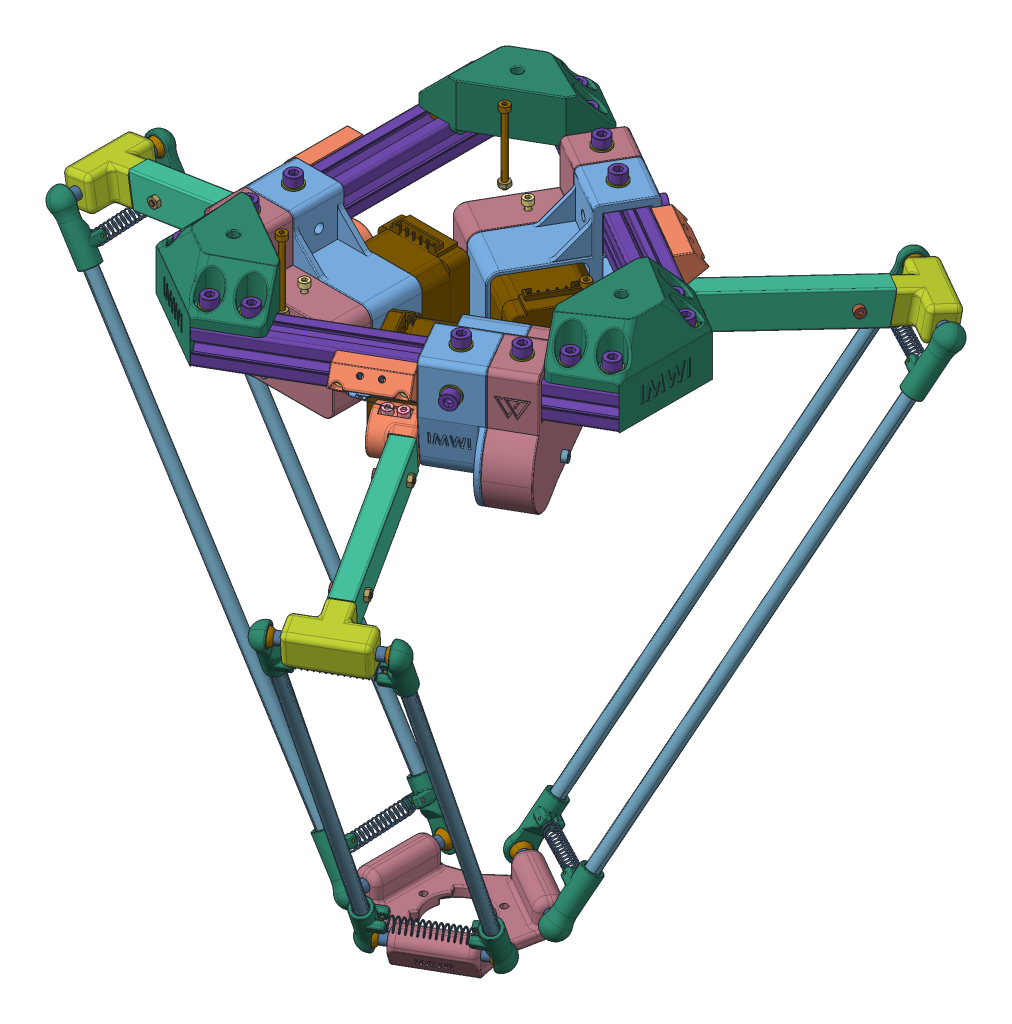
SolidWorks assembly Delta X 1 - v2, configuration 默认. Lengths in mm.
Overall size (365.97 369.79 411.99).
296 component instances, 48 part files, 0 mates.
Components (placement in the parent):
- Delta X 1 - v2.STEP-1: Delta X 1 - v2.STEP [默认] at origin size (365.97 369.79 411.99)
  - Outer Arm.STEP-1: Outer Arm.STEP [默认] at (231.4137 119.905 169.256) x (0.493973 -0.154803 0.855586) z (-0.077402 -0.987945 -0.134064) size (150 86.45 25.5)
    - inox8.STEP-1: inox8.STEP [默认] at (18.6919 -1.6129 59.7906) size (8 70 8)
    - Shoulder.STEP-1: Shoulder.STEP [默认] at (18.6919 46.2871 59.7906) x (0 0 -1) z (0 1 0) size (24 54 22.11)
    - Nut m3.STEP-1: Nut m3.STEP [默认] at (18.6919 61.3871 54.0406) x (0.866025 -0.5 0) z (-0.5 -0.866025 0) size (7.37 2.8 5.8)
    - Nut m3.STEP-2: Nut m3.STEP [默认] at (18.6919 54.3871 54.0406) x (0.99558 -0.093914 0) z (-0.093914 -0.99558 0) size (7.37 2.8 5.8)
    - M3x8 bolt_M3x8 bolt.STEP-1: M3x8 bolt_M3x8 bolt.STEP [默认] at (18.6919 61.3871 46.2906) x (0 0 1) z (-1 0 0) size (11 5.5 5.5)
    - M3x8 bolt_M3x8 bolt.STEP-2: M3x8 bolt_M3x8 bolt.STEP [默认] at (18.6919 54.3871 46.2906) x (0 0 1) z (-1 0 0) size (11 5.5 5.5)
    - ring 8mm.STEP-1: ring 8mm.STEP [默认] at (18.6919 45.2871 59.7906) size (10.45 1 10.45)
    - Nhomtay_Default_As Machined_.STEP-1: Nhomtay_Default_As Machined_.STEP [默认] at (130.6919 51.8371 59.7906) x (0 0 1) z (0 -1 0) size (20 100 12)
    - ElbowV2.STEP-1: ElbowV2.STEP [默认] at (130.6919 51.8371 50.3406) x (0 -1 0) z (0 0 1) size (40 52 18.92)
    - M4x60 thread_M4x60 thread.STEP-1: M4x60 thread_M4x60 thread.STEP [默认] at (148.6919 96.8371 59.7906) x (0 -1 0) z (0 0 1) size (58 4 4)
    - Joint Ball.STEP-1: Joint Ball.STEP [默认] at (148.6919 79.8371 59.7906) x (0 -1 0) z (-0.713634 0 0.700519) size (9 10 10)
    - vongdem3m.STEP-1: vongdem3m.STEP [默认] at (148.6919 71.8371 59.7906) x (0.999724 0 -0.023481) z (0 1 0) size (6.4 6.4 4)
    - Joint Ball.STEP-2: Joint Ball.STEP [默认] at (148.6919 23.8371 59.7906) x (0 1 0) z (0.144688 0 0.989477) size (9 10 10)
    - vongdem3m.STEP-2: vongdem3m.STEP [默认] at (148.6919 27.8371 59.7906) x (0.999724 0 -0.023481) z (0 1 0) size (6.4 6.4 4)
    - M3x15 bolt_M3x8 bolt.STEP-1: M3x15 bolt_M3x8 bolt.STEP [默认] at (45.6919 60.8371 59.7906) x (0 -1 0) z (0 0 1) size (18 5.5 5.5)
    - M3x15 bolt_M3x8 bolt.STEP-2: M3x15 bolt_M3x8 bolt.STEP [默认] at (115.6919 60.8371 59.7906) x (0 -1 0) z (0 0 1) size (18 5.5 5.5)
    - M3 Nut_M3 Nut.STEP-1: M3 Nut_M3 Nut.STEP [默认] at (45.6919 43.4371 59.7906) x (1 0 0) z (0 -1 0) size (5.5 6.35 2.4)
    - M3 Nut_M3 Nut.STEP-2: M3 Nut_M3 Nut.STEP [默认] at (115.6919 43.4371 59.7906) x (1 0 0) z (0 -1 0) size (5.5 6.35 2.4)
  - Outer Arm.STEP-2: Outer Arm.STEP [默认] at (141.6292 119.905 55.839) x (0.493973 -0.154803 -0.855586) z (-0.077402 -0.987945 0.134064) size (150 86.45 25.5)
    - inox8.STEP-1: inox8.STEP [默认] at (18.6919 -1.6129 59.7906) size (8 70 8)
    - Shoulder.STEP-1: Shoulder.STEP [默认] at (18.6919 46.2871 59.7906) x (0 0 -1) z (0 1 0) size (24 54 22.11)
    - Nut m3.STEP-1: Nut m3.STEP [默认] at (18.6919 61.3871 54.0406) x (0.866025 -0.5 0) z (-0.5 -0.866025 0) size (7.37 2.8 5.8)
    - Nut m3.STEP-2: Nut m3.STEP [默认] at (18.6919 54.3871 54.0406) x (0.99558 -0.093914 0) z (-0.093914 -0.99558 0) size (7.37 2.8 5.8)
    - M3x8 bolt_M3x8 bolt.STEP-1: M3x8 bolt_M3x8 bolt.STEP [默认] at (18.6919 61.3871 46.2906) x (0 0 1) z (-1 0 0) size (11 5.5 5.5)
    - M3x8 bolt_M3x8 bolt.STEP-2: M3x8 bolt_M3x8 bolt.STEP [默认] at (18.6919 54.3871 46.2906) x (0 0 1) z (-1 0 0) size (11 5.5 5.5)
    - ring 8mm.STEP-1: ring 8mm.STEP [默认] at (18.6919 45.2871 59.7906) size (10.45 1 10.45)
    - Nhomtay_Default_As Machined_.STEP-1: Nhomtay_Default_As Machined_.STEP [默认] at (130.6919 51.8371 59.7906) x (0 0 1) z (0 -1 0) size (20 100 12)
    - ElbowV2.STEP-1: ElbowV2.STEP [默认] at (130.6919 51.8371 50.3406) x (0 -1 0) z (0 0 1) size (40 52 18.92)
    - M4x60 thread_M4x60 thread.STEP-1: M4x60 thread_M4x60 thread.STEP [默认] at (148.6919 96.8371 59.7906) x (0 -1 0) z (0 0 1) size (58 4 4)
    - Joint Ball.STEP-1: Joint Ball.STEP [默认] at (148.6919 79.8371 59.7906) x (0 -1 0) z (-0.713634 0 0.700519) size (9 10 10)
    - vongdem3m.STEP-1: vongdem3m.STEP [默认] at (148.6919 71.8371 59.7906) x (0.999724 0 -0.023481) z (0 1 0) size (6.4 6.4 4)
    - Joint Ball.STEP-2: Joint Ball.STEP [默认] at (148.6919 23.8371 59.7906) x (0 1 0) z (0.144688 0 0.989477) size (9 10 10)
    - vongdem3m.STEP-2: vongdem3m.STEP [默认] at (148.6919 27.8371 59.7906) x (0.999724 0 -0.023481) z (0 1 0) size (6.4 6.4 4)
    - M3x15 bolt_M3x8 bolt.STEP-1: M3x15 bolt_M3x8 bolt.STEP [默认] at (45.6919 60.8371 59.7906) x (0 -1 0) z (0 0 1) size (18 5.5 5.5)
    - M3x15 bolt_M3x8 bolt.STEP-2: M3x15 bolt_M3x8 bolt.STEP [默认] at (115.6919 60.8371 59.7906) x (0 -1 0) z (0 0 1) size (18 5.5 5.5)
    - M3 Nut_M3 Nut.STEP-1: M3 Nut_M3 Nut.STEP [默认] at (45.6919 43.4371 59.7906) x (1 0 0) z (0 -1 0) size (5.5 6.35 2.4)
    - M3 Nut_M3 Nut.STEP-2: M3 Nut_M3 Nut.STEP [默认] at (115.6919 43.4371 59.7906) x (1 0 0) z (0 -1 0) size (5.5 6.35 2.4)
  - Outer Arm.STEP-3: Outer Arm.STEP [默认] at (88.2995 119.905 190.3032) x (-0.987945 -0.154803 0) z (0.154803 -0.987945 0) size (150 86.45 25.5)
    - inox8.STEP-1: inox8.STEP [默认] at (18.6919 -1.6129 59.7906) size (8 70 8)
    - Shoulder.STEP-1: Shoulder.STEP [默认] at (18.6919 46.2871 59.7906) x (0 0 -1) z (0 1 0) size (24 54 22.11)
    - Nut m3.STEP-1: Nut m3.STEP [默认] at (18.6919 61.3871 54.0406) x (0.866025 -0.5 0) z (-0.5 -0.866025 0) size (7.37 2.8 5.8)
    - Nut m3.STEP-2: Nut m3.STEP [默认] at (18.6919 54.3871 54.0406) x (0.99558 -0.093914 0) z (-0.093914 -0.99558 0) size (7.37 2.8 5.8)
    - M3x8 bolt_M3x8 bolt.STEP-1: M3x8 bolt_M3x8 bolt.STEP [默认] at (18.6919 61.3871 46.2906) x (0 0 1) z (-1 0 0) size (11 5.5 5.5)
    - M3x8 bolt_M3x8 bolt.STEP-2: M3x8 bolt_M3x8 bolt.STEP [默认] at (18.6919 54.3871 46.2906) x (0 0 1) z (-1 0 0) size (11 5.5 5.5)
    - ring 8mm.STEP-1: ring 8mm.STEP [默认] at (18.6919 45.2871 59.7906) size (10.45 1 10.45)
    - Nhomtay_Default_As Machined_.STEP-1: Nhomtay_Default_As Machined_.STEP [默认] at (130.6919 51.8371 59.7906) x (0 0 1) z (0 -1 0) size (20 100 12)
    - ElbowV2.STEP-1: ElbowV2.STEP [默认] at (130.6919 51.8371 50.3406) x (0 -1 0) z (0 0 1) size (40 52 18.92)
    - M4x60 thread_M4x60 thread.STEP-1: M4x60 thread_M4x60 thread.STEP [默认] at (148.6919 96.8371 59.7906) x (0 -1 0) z (0 0 1) size (58 4 4)
    - Joint Ball.STEP-1: Joint Ball.STEP [默认] at (148.6919 79.8371 59.7906) x (0 -1 0) z (-0.713634 0 0.700519) size (9 10 10)
    - vongdem3m.STEP-1: vongdem3m.STEP [默认] at (148.6919 71.8371 59.7906) x (0.999724 0 -0.023481) z (0 1 0) size (6.4 6.4 4)
    - Joint Ball.STEP-2: Joint Ball.STEP [默认] at (148.6919 23.8371 59.7906) x (0 1 0) z (0.144688 0 0.989477) size (9 10 10)
    - vongdem3m.STEP-2: vongdem3m.STEP [默认] at (148.6919 27.8371 59.7906) x (0.999724 0 -0.023481) z (0 1 0) size (6.4 6.4 4)
    - M3x15 bolt_M3x8 bolt.STEP-1: M3x15 bolt_M3x8 bolt.STEP [默认] at (45.6919 60.8371 59.7906) x (0 -1 0) z (0 0 1) size (18 5.5 5.5)
    - M3x15 bolt_M3x8 bolt.STEP-2: M3x15 bolt_M3x8 bolt.STEP [默认] at (115.6919 60.8371 59.7906) x (0 -1 0) z (0 0 1) size (18 5.5 5.5)
    - M3 Nut_M3 Nut.STEP-1: M3 Nut_M3 Nut.STEP [默认] at (45.6919 43.4371 59.7906) x (1 0 0) z (0 -1 0) size (5.5 6.35 2.4)
    - M3 Nut_M3 Nut.STEP-2: M3 Nut_M3 Nut.STEP [默认] at (115.6919 43.4371 59.7906) x (1 0 0) z (0 -1 0) size (5.5 6.35 2.4)
  - MovingBase.STEP-1: MovingBase.STEP [默认] at (35.2258 -322.437 -163.4216) x (0.349728 0 0.936851) z (0 1 0) size (119.04 117.52 20.05)
    - Base-EndEffecterV2.STEP-1: Base-EndEffecterV2.STEP [默认] at (324.2859 5.4897 79.9169) x (0.771299 0.636473 0) z (0 0 1) size (89.65 78.39 20.05)
    - Joint Ball.STEP-1: Joint Ball.STEP [默认] at (338.4028 -36.7562 92.9169) x (-0.936851 0.349728 0) z (-0.29757 -0.79713 0.525391) size (9 10 10)
    - Joint Ball.STEP-2: Joint Ball.STEP [默认] at (285.9391 -17.1714 92.9169) x (0.936851 -0.349728 0) z (0 0 1) size (9 10 10)
    - vongdem3m.STEP-1: vongdem3m.STEP [默认] at (334.6554 -35.3573 92.9169) x (0.106119 0.284272 0.952853) z (-0.936851 0.349728 0) size (6.4 6.4 4)
    - vongdem3m.STEP-2: vongdem3m.STEP [默认] at (293.434 -19.9692 92.9169) x (0.09677 0.259227 0.960956) z (-0.936851 0.349728 0) size (6.4 6.4 4)
    - M4x60 thread_M4x60 thread.STEP-1: M4x60 thread_M4x60 thread.STEP [默认] at (267.5294 3.567 92.9169) x (0.771299 0.636473 0) z (0.59811 -0.72481 -0.341927) size (58 4 4)
    - M4x60 thread_M4x60 thread.STEP-2: M4x60 thread_M4x60 thread.STEP [默认] at (350.9991 55.6036 92.9169) x (0.165552 -0.986201 0) z (-0.926759 -0.155574 -0.341927) size (58 4 4)
    - M4x60 thread_M4x60 thread.STEP-3: M4x60 thread_M4x60 thread.STEP [默认] at (354.3293 -42.7016 92.9169) x (-0.936851 0.349728 0) z (0.328649 0.880384 -0.341927) size (58 4 4)
    - vongdem3m.STEP-3: vongdem3m.STEP [默认] at (283.7267 16.9329 92.9169) x (0.193127 -0.234038 0.952853) z (0.771299 0.636473 0) size (6.4 6.4 4)
    - vongdem3m.STEP-4: vongdem3m.STEP [默认] at (354.4757 34.8934 92.9169) x (-0.299246 -0.050234 0.952853) z (0.165552 -0.986201 0) size (6.4 6.4 4)
    - Joint Ball.STEP-3: Joint Ball.STEP [默认] at (280.6415 14.387 92.9169) x (0.771299 0.636473 0) z (-0.54155 0.656269 0.525391) size (9 10 10)
    - Joint Ball.STEP-4: Joint Ball.STEP [默认] at (353.8135 38.8382 92.9169) x (0.165552 -0.986201 0) z (0.83912 0.140862 0.525391) size (9 10 10)
    - vongdem3m.STEP-5: vongdem3m.STEP [默认] at (317.6638 44.9377 92.9169) x (0.176112 -0.213418 0.960956) z (0.771299 0.636473 0) size (6.4 6.4 4)
    - vongdem3m.STEP-6: vongdem3m.STEP [默认] at (361.76 -8.4994 92.9169) x (-0.272882 -0.045808 0.960956) z (0.165552 -0.986201 0) size (6.4 6.4 4)
    - Joint Ball.STEP-5: Joint Ball.STEP [默认] at (323.8342 50.0295 92.9169) x (-0.771299 -0.636473 0) z (0 0 1) size (9 10 10)
    - Joint Ball.STEP-6: Joint Ball.STEP [默认] at (363.0844 -16.3891 92.9169) x (-0.165552 0.986201 0) z (0 0 1) size (9 10 10)
  - OuterArm1.STEP-1: OuterArm1.STEP [默认] at (-114.8621 147.6011 176.4736) x (0 0 1) z (0.53358 -0.845749 0) size (17.15 14.45 330.3)
    - cacbon.STEP-1: cacbon.STEP [默认] at (-10.0075 3.3175 142.8088) size (7 7 286)
    - RodEnd-1-V2.STEP-1: RodEnd-1-V2.STEP [默认] at (-10.0075 3.3175 443.8088) x (1 0 0) z (0 -1 0) size (17.15 37.15 14.3)
    - Spring Stick.STEP-1: Spring Stick.STEP [默认] at (-17.5075 3.3175 423.8089) size (1.5 11.15 1.5)
    - RodEnd-1-V2.STEP-2: RodEnd-1-V2.STEP [默认] at (-10.0075 3.1669 127.8088) x (1 0 0) z (0 1 0) size (17.15 37.15 14.3)
    - Spring Stick.STEP-2: Spring Stick.STEP [默认] at (-17.5075 3.3175 147.8086) size (1.5 11.15 1.5)
  - OuterArm1.STEP-2: OuterArm1.STEP [默认] at (-120.3462 144.1411 100.4586) x (0 0 -1) z (0.53358 -0.845749 0) size (17.15 14.45 330.3)
    - cacbon.STEP-1: cacbon.STEP [默认] at (-10.0075 3.3175 142.8088) size (7 7 286)
    - RodEnd-1-V2.STEP-1: RodEnd-1-V2.STEP [默认] at (-10.0075 3.3175 443.8088) x (1 0 0) z (0 -1 0) size (17.15 37.15 14.3)
    - Spring Stick.STEP-1: Spring Stick.STEP [默认] at (-17.5075 3.3175 423.8089) size (1.5 11.15 1.5)
    - RodEnd-1-V2.STEP-2: RodEnd-1-V2.STEP [默认] at (-10.0075 3.1669 127.8088) x (1 0 0) z (0 1 0) size (17.15 37.15 14.3)
    - Spring Stick.STEP-2: Spring Stick.STEP [默认] at (-17.5075 3.3175 147.8086) size (1.5 11.15 1.5)
  - OuterArm1.STEP-3: OuterArm1.STEP [默认] at (257.9288 144.1411 394.8708) x (-0.866025 0 0.5) z (-0.26679 -0.845749 -0.462094) size (17.15 14.45 330.3)
    - cacbon.STEP-1: cacbon.STEP [默认] at (-10.0075 3.3175 142.8088) size (7 7 286)
    - RodEnd-1-V2.STEP-1: RodEnd-1-V2.STEP [默认] at (-10.0075 3.3175 443.8088) x (1 0 0) z (0 -1 0) size (17.15 37.15 14.3)
    - Spring Stick.STEP-1: Spring Stick.STEP [默认] at (-17.5075 3.3175 423.8089) size (1.5 11.15 1.5)
    - RodEnd-1-V2.STEP-2: RodEnd-1-V2.STEP [默认] at (-10.0075 3.1669 127.8088) x (1 0 0) z (0 1 0) size (17.15 37.15 14.3)
    - Spring Stick.STEP-2: Spring Stick.STEP [默认] at (-17.5075 3.3175 147.8086) size (1.5 11.15 1.5)
  - OuterArm1.STEP-4: OuterArm1.STEP [默认] at (323.7598 144.1411 -79.9311) x (0.866025 0 0.5) z (-0.26679 -0.845749 0.462094) size (17.15 14.45 330.3)
    - cacbon.STEP-1: cacbon.STEP [默认] at (-10.0075 3.3175 142.8088) size (7 7 286)
    - RodEnd-1-V2.STEP-1: RodEnd-1-V2.STEP [默认] at (-10.0075 3.3175 443.8088) x (1 0 0) z (0 -1 0) size (17.15 37.15 14.3)
    - Spring Stick.STEP-1: Spring Stick.STEP [默认] at (-17.5075 3.3175 423.8089) size (1.5 11.15 1.5)
    - RodEnd-1-V2.STEP-2: RodEnd-1-V2.STEP [默认] at (-10.0075 3.1669 127.8088) x (1 0 0) z (0 1 0) size (17.15 37.15 14.3)
    - Spring Stick.STEP-2: Spring Stick.STEP [默认] at (-17.5075 3.3175 147.8086) size (1.5 11.15 1.5)
  - OuterArm1.STEP-5: OuterArm1.STEP [默认] at (321.0177 147.6011 352.1139) x (0.866025 0 -0.5) z (-0.26679 -0.845749 -0.462094) size (17.15 14.45 330.3)
    - cacbon.STEP-1: cacbon.STEP [默认] at (-10.0075 3.3175 142.8088) size (7 7 286)
    - RodEnd-1-V2.STEP-1: RodEnd-1-V2.STEP [默认] at (-10.0075 3.3175 443.8088) x (1 0 0) z (0 -1 0) size (17.15 37.15 14.3)
    - Spring Stick.STEP-1: Spring Stick.STEP [默认] at (-17.5075 3.3175 423.8089) size (1.5 11.15 1.5)
    - RodEnd-1-V2.STEP-2: RodEnd-1-V2.STEP [默认] at (-10.0075 3.1669 127.8088) x (1 0 0) z (0 1 0) size (17.15 37.15 14.3)
    - Spring Stick.STEP-2: Spring Stick.STEP [默认] at (-17.5075 3.3175 147.8086) size (1.5 11.15 1.5)
  - OuterArm1.STEP-6: OuterArm1.STEP [默认] at (255.1868 147.6011 -113.1892) x (-0.866025 0 -0.5) z (-0.26679 -0.845749 0.462094) size (17.15 14.45 330.3)
    - cacbon.STEP-1: cacbon.STEP [默认] at (-10.0075 3.3175 142.8088) size (7 7 286)
    - RodEnd-1-V2.STEP-1: RodEnd-1-V2.STEP [默认] at (-10.0075 3.3175 443.8088) x (1 0 0) z (0 -1 0) size (17.15 37.15 14.3)
    - Spring Stick.STEP-1: Spring Stick.STEP [默认] at (-17.5075 3.3175 423.8089) size (1.5 11.15 1.5)
    - RodEnd-1-V2.STEP-2: RodEnd-1-V2.STEP [默认] at (-10.0075 3.1669 127.8088) x (1 0 0) z (0 1 0) size (17.15 37.15 14.3)
    - Spring Stick.STEP-2: Spring Stick.STEP [默认] at (-17.5075 3.3175 147.8086) size (1.5 11.15 1.5)
  - 2020_Alu profile_Default_As Machined_.STEP-1: 2020_Alu profile_Default_As Machined_.STEP [默认] at (79.0887 91.9416 230.5161) size (20 20 184)
  - Stepper Servo.STEP-1: Stepper Servo.STEP [默认] at (116.6887 57.9416 115.0161) x (-1 0 0) z (0 0 1) size (42.5 46.75 68)
  - GearboxBody V2.STEP-1: GearboxBody V2.STEP [默认] at (79.0887 91.9416 170.0161) size (85.85 74.01 30.29)
  - Alu plate increase hardness.STEP-1: Alu plate increase hardness.STEP [默认] at (79.0887 57.9416 178.0161) x (1 0 0) z (0 1 0) size (80 3 44.3)
  - Cross M3x10 bolt_Cross M3x10 bolt.STEP-1: Cross M3x10 bolt_Cross M3x10 bolt.STEP [默认] at (79.0887 39.3666 179.4161) x (0 0 -1) z (-0.923728 -0.383049 0) size (10 5.5 5.5)
  - Cross M3x10 bolt_Cross M3x10 bolt.STEP-2: Cross M3x10 bolt_Cross M3x10 bolt.STEP [默认] at (79.0887 76.5166 179.4161) x (0 0 -1) z (-0.280639 0.959813 0) size (10 5.5 5.5)
  - M3 Nut_M3 Nut.STEP-1: M3 Nut_M3 Nut.STEP [默认] at (79.0887 76.5166 169.6161) x (0.5 0.866025 0) z (0 0 -1) size (5.5 6.35 2.4)
  - M3 Nut_M3 Nut.STEP-2: M3 Nut_M3 Nut.STEP [默认] at (79.0887 39.3666 169.6161) x (0.5 0.866025 0) z (0 0 -1) size (5.5 6.35 2.4)
  - Bearing 8_16.STEP-1: Bearing 8_16.STEP [默认] at (79.0887 57.9416 172.5161) x (0.889226 0.457467 0) z (0 0 1) size (16 16 5)
  - Bearing 8_16.STEP-2: Bearing 8_16.STEP [默认] at (79.0887 57.9416 147.5161) x (-0.986457 0.164017 0) z (0 0 1) size (16 16 5)
  - Bearing 5_16.STEP-1: Bearing 5_16.STEP [默认] at (107.7439 45.7053 186.7661) x (-0.939098 0.34365 0) z (0 0 1) size (11 11 5)
  - BeltTensioner.STEP-1: BeltTensioner.STEP [默认] at (122.1887 44.4416 192.1661) x (0.999848 0.017452 0) z (0 0 1) size (32.71 12.76 9.8)
  - BeltTensioner2.STEP-1: BeltTensioner2.STEP [默认] at (122.1887 44.4416 192.1661) x (0.999848 0.017452 0) z (0 0 1) size (32.71 12.76 9.8)
  - BeltTensionerBase-v1.STEP-1: BeltTensionerBase-v1.STEP [默认] at (127.3887 57.4416 175.0161) x (0 1 0) z (1 0 0) size (40.1 16.43 24.55)
  - Cross M3x16 bolt_Cross M3x10 bolt.STEP-1: Cross M3x16 bolt_Cross M3x10 bolt.STEP [默认] at (132.1887 42.4416 181.4161) x (0 0 -1) z (0.065564 -0.997848 0) size (16 5.5 5.5)
  - M3x25 bolt_M3x8 bolt.STEP-1: M3x25 bolt_M3x8 bolt.STEP [默认] at (132.1887 73.4416 194.4161) x (0 0 -1) z (1 0 0) size (28 5.5 5.5)
  - M3x12 bolt_M3x8 bolt.STEP-1: M3x12 bolt_M3x8 bolt.STEP [默认] at (107.7439 45.7053 194.6661) x (0 0 -1) z (1 0 0) size (15 5.5 5.5)
  - M3 Nut_M3 Nut.STEP-3: M3 Nut_M3 Nut.STEP [默认] at (107.7439 45.7053 179.4661) x (0.5 0.866025 0) z (0 0 -1) size (5.5 6.35 2.4)
  - M3x20 bolt_M3x8 bolt.STEP-1: M3x20 bolt_M3x8 bolt.STEP [默认] at (122.1887 44.4416 194.6661) x (0 0 -1) z (1 0 0) size (23 5.5 5.5)
  - ring 8mm.STEP-1: ring 8mm.STEP [默认] at (79.0887 57.9416 175.0161) x (1 0 0) z (0 -1 0) size (10.45 1 10.45)
  - GearboxLid V2.STEP-1: GearboxLid V2.STEP [默认] at (79.0887 91.9416 195.4161) size (85.85 74 22.42)
  - M3 Nut_M3 Nut.STEP-4: M3 Nut_M3 Nut.STEP [默认] at (110.9759 77.0916 185.4195) x (1 0 0) z (0 1 0) size (5.5 6.35 2.4)
  - M3x30 bolt_M3x8 bolt.STEP-1: M3x30 bolt_M3x8 bolt.STEP [默认] at (101.1887 42.4416 200.4161) x (0 0 -1) z (1 0 0) size (33 5.5 5.5)
  - M3x30 bolt_M3x8 bolt.STEP-2: M3x30 bolt_M3x8 bolt.STEP [默认] at (101.1887 73.4416 200.4161) x (0 0 -1) z (1 0 0) size (33 5.5 5.5)
  - Frame connector.STEP-1: Frame connector.STEP [默认] at (97.7489 101.9416 235.5161) x (0.866025 0 0.5) z (0 -1 0) size (84.39 40.74 45.28)
  - M5 Washer_M5 Washer.STEP-1: M5 Washer_M5 Washer.STEP [默认] at (131.8474 107.0381 237.3764) x (0 1 0) z (0 0 1) size (1 10 10)
  - M5 Washer_M5 Washer.STEP-2: M5 Washer_M5 Washer.STEP [默认] at (116.2589 106.9416 246.3764) x (0 -1 0) z (0 0 1) size (1 10 10)
  - M5 Washer_M5 Washer.STEP-3: M5 Washer_M5 Washer.STEP [默认] at (79.0887 106.9416 224.9161) x (0 -1 0) z (0 0 1) size (1 10 10)
  - M5 Washer_M5 Washer.STEP-4: M5 Washer_M5 Washer.STEP [默认] at (79.0887 106.9416 206.9161) x (0 -1 0) z (0 0 1) size (1 10 10)
  - M5 Washer_M5 Washer.STEP-5: M5 Washer_M5 Washer.STEP [默认] at (79.0887 106.9416 186.2161) x (0 -1 0) z (0 0 1) size (1 10 10)
  - M5 Washer_M5 Washer.STEP-6: M5 Washer_M5 Washer.STEP [默认] at (79.0887 106.9416 160.0161) x (0 -1 0) z (0.543109 0 -0.839662) size (1 10 10)
  - M5 Washer_M5 Washer.STEP-7: M5 Washer_M5 Washer.STEP [默认] at (64.0887 91.9416 160.0161) size (1 10 10)
  - M5x10 bolt_M5x10 bolt.STEP-1: M5x10 bolt_M5x10 bolt.STEP [默认] at (79.0887 112.9416 224.9161) x (0 -1 0) z (0 0 1) size (15 8.5 8.5)
  - M5x10 bolt_M5x10 bolt.STEP-2: M5x10 bolt_M5x10 bolt.STEP [默认] at (79.0887 112.9416 206.9161) x (0 -1 0) z (0 0 1) size (15 8.5 8.5)
  - M5x10 bolt_M5x10 bolt.STEP-3: M5x10 bolt_M5x10 bolt.STEP [默认] at (79.0887 112.9416 186.2161) x (0 -1 0) z (0 0 1) size (15 8.5 8.5)
  - M5x10 bolt_M5x10 bolt.STEP-4: M5x10 bolt_M5x10 bolt.STEP [默认] at (79.0887 112.9416 160.0161) x (0 -1 0) z (0 0 1) size (15 8.5 8.5)
  - M5x10 bolt_M5x10 bolt.STEP-5: M5x10 bolt_M5x10 bolt.STEP [默认] at (58.0887 91.9416 160.0161) size (15 8.5 8.5)
  - M5x10 bolt_M5x10 bolt.STEP-6: M5x10 bolt_M5x10 bolt.STEP [默认] at (116.2589 112.9416 246.3764) x (0 -1 0) z (0 0 1) size (15 8.5 8.5)
  - M5x10 bolt_M5x10 bolt.STEP-7: M5x10 bolt_M5x10 bolt.STEP [默认] at (131.8474 112.0381 237.3764) x (0 -1 0) z (0 0 1) size (15 8.5 8.5)
  - T Slot Nut_______ _______ 6__ _5.STEP-1: T Slot Nut_______ _______ 6__ _5.STEP [默认] at (79.0887 97.2416 155.0161) size (9.4 4.5 10)
  - T Slot Nut_______ _______ 6__ _5.STEP-2: T Slot Nut_______ _______ 6__ _5.STEP [默认] at (73.7887 91.9416 155.0161) x (0 1 0) z (0 0 1) size (9.4 4.5 10)
  - T Slot Nut_______ _______ 6__ _5.STEP-3: T Slot Nut_______ _______ 6__ _5.STEP [默认] at (79.0887 97.2416 181.2161) size (9.4 4.5 10)
  - T Slot Nut_______ _______ 6__ _5.STEP-4: T Slot Nut_______ _______ 6__ _5.STEP [默认] at (79.0887 97.2416 201.0161) size (9.4 4.5 10)
  - T Slot Nut_______ _______ 6__ _5.STEP-5: T Slot Nut_______ _______ 6__ _5.STEP [默认] at (79.0887 97.2416 219.0161) size (9.4 4.5 10)
  - T Slot Nut_______ _______ 6__ _5.STEP-6: T Slot Nut_______ _______ 6__ _5.STEP [默认] at (128.2967 97.2416 239.4263) x (-0.5 0 -0.866025) z (0.866025 0 -0.5) size (9.4 4.5 10)
  - T Slot Nut_______ _______ 6__ _5.STEP-7: T Slot Nut_______ _______ 6__ _5.STEP [默认] at (112.7082 97.2416 248.4263) x (-0.5 0 -0.866025) z (0.866025 0 -0.5) size (9.4 4.5 10)
  - M3 Nut_M3 Nut.STEP-5: M3 Nut_M3 Nut.STEP [默认] at (212.3063 45.7053 157.8352) x (-0.25 0.866025 -0.433013) z (-0.866025 0 0.5) size (5.5 6.35 2.4)
  - M3 Nut_M3 Nut.STEP-6: M3 Nut_M3 Nut.STEP [默认] at (141.2922 45.7053 78.097) x (-0.25 0.866025 0.433013) z (0.866025 0 0.5) size (5.5 6.35 2.4)
  - Stepper Servo.STEP-2: Stepper Servo.STEP [默认] at (152.0185 57.9416 182.3138) x (0.5 0 0.866025) z (0.866025 0 -0.5) size (42.5 46.75 68)
  - Stepper Servo.STEP-3: Stepper Servo.STEP [默认] at (192.6351 57.9416 118.0684) x (0.5 0 -0.866025) z (-0.866025 0 -0.5) size (42.5 46.75 68)
  - Cross M3x10 bolt_Cross M3x10 bolt.STEP-3: Cross M3x10 bolt_Cross M3x10 bolt.STEP [默认] at (226.5906 76.5166 182.6764) x (-0.866025 0 0.5) z (0.14032 0.959813 0.243041) size (10 5.5 5.5)
  - Cross M3x10 bolt_Cross M3x10 bolt.STEP-4: Cross M3x10 bolt_Cross M3x10 bolt.STEP [默认] at (155.6631 76.5166 53.3058) x (0.866025 0 0.5) z (0.14032 0.959813 -0.243041) size (10 5.5 5.5)
  - T Slot Nut_______ _______ 6__ _5.STEP-8: T Slot Nut_______ _______ 6__ _5.STEP [默认] at (228.1494 97.2416 181.7764) x (-0.5 0 -0.866025) z (0.866025 0 -0.5) size (9.4 4.5 10)
  - T Slot Nut_______ _______ 6__ _5.STEP-9: T Slot Nut_______ _______ 6__ _5.STEP [默认] at (154.1043 97.2416 52.4058) x (-0.5 0 0.866025) z (-0.866025 0 -0.5) size (9.4 4.5 10)
  - T Slot Nut_______ _______ 6__ _5.STEP-10: T Slot Nut_______ _______ 6__ _5.STEP [默认] at (208.1096 91.9416 199.4663) x (0 1 0) z (0.866025 0 -0.5) size (9.4 4.5 10)
  - T Slot Nut_______ _______ 6__ _5.STEP-11: T Slot Nut_______ _______ 6__ _5.STEP [默认] at (179.4441 91.9416 60.9159) x (0 1 0) z (-0.866025 0 -0.5) size (9.4 4.5 10)
  - T Slot Nut_______ _______ 6__ _5.STEP-12: T Slot Nut_______ _______ 6__ _5.STEP [默认] at (260.8852 97.2416 162.8764) x (-0.5 0 -0.866025) z (0.866025 0 -0.5) size (9.4 4.5 10)
  - T Slot Nut_______ _______ 6__ _5.STEP-13: T Slot Nut_______ _______ 6__ _5.STEP [默认] at (121.3685 97.2416 33.5058) x (-0.5 0 0.866025) z (-0.866025 0 -0.5) size (9.4 4.5 10)
  - T Slot Nut_______ _______ 6__ _5.STEP-14: T Slot Nut_______ _______ 6__ _5.STEP [默认] at (253.957 97.2416 110.0558) x (-0.5 0 0.866025) z (-0.866025 0 -0.5) size (9.4 4.5 10)
  - T Slot Nut_______ _______ 6__ _5.STEP-15: T Slot Nut_______ _______ 6__ _5.STEP [默认] at (79.0887 97.2416 65.9161) size (9.4 4.5 10)
  - T Slot Nut_______ _______ 6__ _5.STEP-16: T Slot Nut_______ _______ 6__ _5.STEP [默认] at (269.5454 97.2416 119.0558) x (-0.5 0 0.866025) z (-0.866025 0 -0.5) size (9.4 4.5 10)
  - T Slot Nut_______ _______ 6__ _5.STEP-17: T Slot Nut_______ _______ 6__ _5.STEP [默认] at (79.0887 97.2416 47.9161) size (9.4 4.5 10)
  - T Slot Nut_______ _______ 6__ _5.STEP-18: T Slot Nut_______ _______ 6__ _5.STEP [默认] at (245.2967 97.2416 171.8764) x (-0.5 0 -0.866025) z (0.866025 0 -0.5) size (9.4 4.5 10)
  - T Slot Nut_______ _______ 6__ _5.STEP-19: T Slot Nut_______ _______ 6__ _5.STEP [默认] at (136.9569 97.2416 42.5058) x (-0.5 0 0.866025) z (-0.866025 0 -0.5) size (9.4 4.5 10)
  - BeltTensionerBase-v1.STEP-2: BeltTensionerBase-v1.STEP [默认] at (198.6301 57.4416 143.0473) x (0 1 0) z (-0.5 0 -0.866025) size (40.1 16.43 24.55)
  - BeltTensionerBase-v1.STEP-3: BeltTensionerBase-v1.STEP [默认] at (135.3236 57.4416 97.3349) x (0 1 0) z (-0.5 0 0.866025) size (40.1 16.43 24.55)
  - Alu plate increase hardness.STEP-2: Alu plate increase hardness.STEP [默认] at (225.3781 57.9416 183.3764) x (-0.5 0 -0.866025) z (0 1 0) size (80 3 44.3)
  - Alu plate increase hardness.STEP-3: Alu plate increase hardness.STEP [默认] at (156.8755 57.9416 54.0058) x (-0.5 0 0.866025) z (0 1 0) size (80 3 44.3)
  - M3x20 bolt_M3x8 bolt.STEP-2: M3x20 bolt_M3x8 bolt.STEP [默认] at (218.2475 44.4416 137.7257) x (-0.866025 0 0.5) z (-0.5 0 -0.866025) size (23 5.5 5.5)
  - M3x20 bolt_M3x8 bolt.STEP-3: M3x20 bolt_M3x8 bolt.STEP [默认] at (120.9062 44.4416 83.0065) x (0.866025 0 0.5) z (-0.5 0 0.866025) size (23 5.5 5.5)
  - M3x12 bolt_M3x8 bolt.STEP-2: M3x12 bolt_M3x8 bolt.STEP [默认] at (225.4699 45.7053 150.2352) x (-0.866025 0 0.5) z (-0.5 0 -0.866025) size (15 5.5 5.5)
  - M3x12 bolt_M3x8 bolt.STEP-3: M3x12 bolt_M3x8 bolt.STEP [默认] at (128.1286 45.7053 70.497) x (0.866025 0 0.5) z (-0.5 0 0.866025) size (15 5.5 5.5)
  - GearboxLid V2.STEP-2: GearboxLid V2.STEP [默认] at (240.447 91.9416 174.6764) x (-0.5 0 -0.866025) z (0.866025 0 -0.5) size (85.85 74 22.42)
  - GearboxLid V2.STEP-3: GearboxLid V2.STEP [默认] at (141.8067 91.9416 45.3058) x (-0.5 0 0.866025) z (-0.866025 0 -0.5) size (85.85 74 22.42)
  - ring 8mm.STEP-2: ring 8mm.STEP [默认] at (222.7801 57.9416 184.8764) x (-0.5 0 -0.866025) z (0 -1 0) size (10.45 1 10.45)
  - ring 8mm.STEP-3: ring 8mm.STEP [默认] at (159.4736 57.9416 55.5058) x (-0.5 0 0.866025) z (0 -1 0) size (10.45 1 10.45)
  - Cross M3x10 bolt_Cross M3x10 bolt.STEP-5: Cross M3x10 bolt_Cross M3x10 bolt.STEP [默认] at (226.5906 39.3666 182.6764) x (-0.866025 0 0.5) z (0.461864 -0.383049 0.799972) size (10 5.5 5.5)
  - Cross M3x10 bolt_Cross M3x10 bolt.STEP-6: Cross M3x10 bolt_Cross M3x10 bolt.STEP [默认] at (155.6631 39.3666 53.3058) x (0.866025 0 0.5) z (0.461864 -0.383049 -0.799972) size (10 5.5 5.5)
  - Cross M3x16 bolt_Cross M3x10 bolt.STEP-2: Cross M3x16 bolt_Cross M3x10 bolt.STEP [默认] at (201.7726 42.4416 135.6904) x (-0.866025 0 0.5) z (-0.032782 -0.997848 -0.05678) size (16 5.5 5.5)
  - Cross M3x16 bolt_Cross M3x10 bolt.STEP-3: Cross M3x16 bolt_Cross M3x10 bolt.STEP [默认] at (127.381 42.4416 98.2918) x (0.866025 0 0.5) z (-0.032782 -0.997848 0.05678) size (16 5.5 5.5)
  - GearboxBody V2.STEP-2: GearboxBody V2.STEP [默认] at (218.4499 91.9416 187.3764) x (-0.5 0 -0.866025) z (0.866025 0 -0.5) size (85.85 74.01 30.29)
  - GearboxBody V2.STEP-3: GearboxBody V2.STEP [默认] at (163.8037 91.9416 58.0058) x (-0.5 0 0.866025) z (-0.866025 0 -0.5) size (85.85 74.01 30.29)
  - M3 Nut_M3 Nut.STEP-7: M3 Nut_M3 Nut.STEP [默认] at (218.1035 39.3666 187.5764) x (-0.25 0.866025 -0.433013) z (-0.866025 0 0.5) size (5.5 6.35 2.4)
  - M3 Nut_M3 Nut.STEP-8: M3 Nut_M3 Nut.STEP [默认] at (164.1501 39.3666 58.2058) x (-0.25 0.866025 0.433013) z (0.866025 0 0.5) size (5.5 6.35 2.4)
  - BeltTensioner2.STEP-2: BeltTensioner2.STEP [默认] at (216.0824 44.4416 138.9757) x (-0.499924 0.017452 -0.865894) z (0.866025 0 -0.5) size (32.71 12.76 9.8)
  - BeltTensioner2.STEP-3: BeltTensioner2.STEP [默认] at (123.0713 44.4416 84.2565) x (-0.499924 0.017452 0.865894) z (-0.866025 0 -0.5) size (32.71 12.76 9.8)
  - M3 Nut_M3 Nut.STEP-9: M3 Nut_M3 Nut.STEP [默认] at (218.1035 76.5166 187.5764) x (-0.25 0.866025 -0.433013) z (-0.866025 0 0.5) size (5.5 6.35 2.4)
  - M3 Nut_M3 Nut.STEP-10: M3 Nut_M3 Nut.STEP [默认] at (164.1501 76.5166 58.2058) x (-0.25 0.866025 0.433013) z (0.866025 0 0.5) size (5.5 6.35 2.4)
  - BeltTensioner.STEP-2: BeltTensioner.STEP [默认] at (216.0824 44.4416 138.9757) x (-0.499924 0.017452 -0.865894) z (0.866025 0 -0.5) size (32.71 12.76 9.8)
  - BeltTensioner.STEP-3: BeltTensioner.STEP [默认] at (123.0713 44.4416 84.2565) x (-0.499924 0.017452 0.865894) z (-0.866025 0 -0.5) size (32.71 12.76 9.8)
  - Bearing 5_16.STEP-2: Bearing 5_16.STEP [默认] at (218.6283 45.7053 154.1852) x (0.469549 0.34365 0.813283) z (0.866025 0 -0.5) size (11 11 5)
  - Bearing 5_16.STEP-3: Bearing 5_16.STEP [默认] at (134.9702 45.7053 74.447) x (0.469549 0.34365 -0.813283) z (-0.866025 0 -0.5) size (11 11 5)
  - M3x25 bolt_M3x8 bolt.STEP-2: M3x25 bolt_M3x8 bolt.STEP [默认] at (213.031 73.4416 129.1904) x (-0.866025 0 0.5) z (-0.5 0 -0.866025) size (28 5.5 5.5)
  - M3x25 bolt_M3x8 bolt.STEP-3: M3x25 bolt_M3x8 bolt.STEP [默认] at (116.1227 73.4416 91.7918) x (0.866025 0 0.5) z (-0.5 0 0.866025) size (28 5.5 5.5)
  - M3x30 bolt_M3x8 bolt.STEP-3: M3x30 bolt_M3x8 bolt.STEP [默认] at (233.7271 73.4416 153.0372) x (-0.866025 0 0.5) z (-0.5 0 -0.866025) size (33 5.5 5.5)
  - M3x30 bolt_M3x8 bolt.STEP-4: M3x30 bolt_M3x8 bolt.STEP [默认] at (126.4266 73.4416 61.945) x (0.866025 0 0.5) z (-0.5 0 0.866025) size (33 5.5 5.5)
  - 2020_Alu profile_Default_As Machined_.STEP-2: 2020_Alu profile_Default_As Machined_.STEP [默认] at (270.8445 91.9416 157.1264) x (-0.5 0 -0.866025) z (0.866025 0 -0.5) size (20 20 184)
  - 2020_Alu profile_Default_As Machined_.STEP-3: 2020_Alu profile_Default_As Machined_.STEP [默认] at (111.4092 91.9416 27.7558) x (-0.5 0 0.866025) z (-0.866025 0 -0.5) size (20 20 184)
  - Bearing 8_16.STEP-3: Bearing 8_16.STEP [默认] at (220.615 57.9416 186.1264) x (-0.444613 0.457467 -0.770093) z (0.866025 0 -0.5) size (16 16 5)
  - Bearing 8_16.STEP-4: Bearing 8_16.STEP [默认] at (161.6387 57.9416 56.7558) x (-0.444613 0.457467 0.770093) z (-0.866025 0 -0.5) size (16 16 5)
  - Bearing 8_16.STEP-5: Bearing 8_16.STEP [默认] at (198.9644 57.9416 198.6264) x (0.493229 0.164017 0.854297) z (0.866025 0 -0.5) size (16 16 5)
  - Bearing 8_16.STEP-6: Bearing 8_16.STEP [默认] at (183.2893 57.9416 69.2558) x (0.493229 0.164017 -0.854297) z (-0.866025 0 -0.5) size (16 16 5)
  - M5 Washer_M5 Washer.STEP-8: M5 Washer_M5 Washer.STEP [默认] at (265.9947 106.9416 117.0058) x (0 -1 0) z (0.866025 0 -0.5) size (1 10 10)
  - M5 Washer_M5 Washer.STEP-9: M5 Washer_M5 Washer.STEP [默认] at (79.0887 106.9416 52.0161) x (0 -1 0) z (-0.866025 0 -0.5) size (1 10 10)
  - M5 Washer_M5 Washer.STEP-10: M5 Washer_M5 Washer.STEP [默认] at (265.9947 106.9416 159.9264) x (0 -1 0) z (0.866025 0 -0.5) size (1 10 10)
  - M5 Washer_M5 Washer.STEP-11: M5 Washer_M5 Washer.STEP [默认] at (116.2589 106.9416 30.5558) x (0 -1 0) z (-0.866025 0 -0.5) size (1 10 10)
  - M5 Washer_M5 Washer.STEP-12: M5 Washer_M5 Washer.STEP [默认] at (250.4063 107.0381 108.0058) x (0 1 0) z (0.866025 0 -0.5) size (1 10 10)
  - M5 Washer_M5 Washer.STEP-13: M5 Washer_M5 Washer.STEP [默认] at (79.0887 107.0381 70.0161) x (0 1 0) z (-0.866025 0 -0.5) size (1 10 10)
  - M5 Washer_M5 Washer.STEP-14: M5 Washer_M5 Washer.STEP [默认] at (209.7897 106.9416 192.3764) x (0 -1 0) z (-0.998723 0 -0.050515) size (1 10 10)
  - M5 Washer_M5 Washer.STEP-15: M5 Washer_M5 Washer.STEP [默认] at (172.464 106.9416 63.0058) x (0 -1 0) z (0.455615 0 0.890177) size (1 10 10)
  - M5 Washer_M5 Washer.STEP-16: M5 Washer_M5 Washer.STEP [默认] at (232.4795 106.9416 179.2764) x (0 -1 0) z (0.866025 0 -0.5) size (1 10 10)
  - M5 Washer_M5 Washer.STEP-17: M5 Washer_M5 Washer.STEP [默认] at (149.7741 106.9416 49.9058) x (0 -1 0) z (-0.866025 0 -0.5) size (1 10 10)
  - M5 Washer_M5 Washer.STEP-18: M5 Washer_M5 Washer.STEP [默认] at (217.2897 91.9416 205.3667) x (-0.5 0 -0.866025) z (0.866025 0 -0.5) size (1 10 10)
  - M5 Washer_M5 Washer.STEP-19: M5 Washer_M5 Washer.STEP [默认] at (179.964 91.9416 50.0155) x (-0.5 0 0.866025) z (-0.866025 0 -0.5) size (1 10 10)
  - M5 Washer_M5 Washer.STEP-20: M5 Washer_M5 Washer.STEP [默认] at (250.4063 106.9416 168.9264) x (0 -1 0) z (0.866025 0 -0.5) size (1 10 10)
  - M5 Washer_M5 Washer.STEP-21: M5 Washer_M5 Washer.STEP [默认] at (131.8474 106.9416 39.5558) x (0 -1 0) z (-0.866025 0 -0.5) size (1 10 10)
  - M3x30 bolt_M3x8 bolt.STEP-5: M3x30 bolt_M3x8 bolt.STEP [默认] at (233.7271 42.4416 153.0372) x (-0.866025 0 0.5) z (-0.5 0 -0.866025) size (33 5.5 5.5)
  - M3x30 bolt_M3x8 bolt.STEP-6: M3x30 bolt_M3x8 bolt.STEP [默认] at (126.4266 42.4416 61.945) x (0.866025 0 0.5) z (-0.5 0 0.866025) size (33 5.5 5.5)
  - M5x10 bolt_M5x10 bolt.STEP-8: M5x10 bolt_M5x10 bolt.STEP [默认] at (250.4063 112.0381 108.0058) x (0 -1 0) z (0.866025 0 -0.5) size (15 8.5 8.5)
  - M5x10 bolt_M5x10 bolt.STEP-9: M5x10 bolt_M5x10 bolt.STEP [默认] at (79.0887 112.0381 70.0161) x (0 -1 0) z (-0.866025 0 -0.5) size (15 8.5 8.5)
  - Frame connector.STEP-2: Frame connector.STEP [默认] at (265.8445 101.9416 138.4661) x (0 0 -1) z (0 -1 0) size (84.39 40.74 45.28)
  - Frame connector.STEP-3: Frame connector.STEP [默认] at (97.7489 101.9416 41.4161) x (-0.866025 0 0.5) z (0 -1 0) size (84.39 40.74 45.28)
  - M3 Nut_M3 Nut.STEP-11: M3 Nut_M3 Nut.STEP [默认] at (215.8461 77.0916 152.0596) x (-0.5 0 -0.866025) z (0 1 0) size (5.5 6.35 2.4)
  - M3 Nut_M3 Nut.STEP-12: M3 Nut_M3 Nut.STEP [默认] at (134.5204 77.0916 77.9193) x (-0.5 0 0.866025) z (0 1 0) size (5.5 6.35 2.4)
  - T Slot Nut_______ _______ 6__ _5.STEP-20: T Slot Nut_______ _______ 6__ _5.STEP [默认] at (205.4596 97.2416 194.8764) x (-0.5 0 -0.866025) z (0.866025 0 -0.5) size (9.4 4.5 10)
  - T Slot Nut_______ _______ 6__ _5.STEP-21: T Slot Nut_______ _______ 6__ _5.STEP [默认] at (176.7941 97.2416 65.5058) x (-0.5 0 0.866025) z (-0.866025 0 -0.5) size (9.4 4.5 10)
  - M5x10 bolt_M5x10 bolt.STEP-10: M5x10 bolt_M5x10 bolt.STEP [默认] at (220.2897 91.9416 210.5629) x (-0.5 0 -0.866025) z (0.866025 0 -0.5) size (15 8.5 8.5)
  - M5x10 bolt_M5x10 bolt.STEP-11: M5x10 bolt_M5x10 bolt.STEP [默认] at (182.964 91.9416 44.8193) x (-0.5 0 0.866025) z (-0.866025 0 -0.5) size (15 8.5 8.5)
  - M5x10 bolt_M5x10 bolt.STEP-12: M5x10 bolt_M5x10 bolt.STEP [默认] at (265.9947 112.9416 117.0058) x (0 -1 0) z (0.866025 0 -0.5) size (15 8.5 8.5)
  - M5x10 bolt_M5x10 bolt.STEP-13: M5x10 bolt_M5x10 bolt.STEP [默认] at (79.0887 112.9416 52.0161) x (0 -1 0) z (-0.866025 0 -0.5) size (15 8.5 8.5)
  - M5x10 bolt_M5x10 bolt.STEP-14: M5x10 bolt_M5x10 bolt.STEP [默认] at (209.7897 112.9416 192.3764) x (0 -1 0) z (0.866025 0 -0.5) size (15 8.5 8.5)
  - M5x10 bolt_M5x10 bolt.STEP-15: M5x10 bolt_M5x10 bolt.STEP [默认] at (172.464 112.9416 63.0058) x (0 -1 0) z (-0.866025 0 -0.5) size (15 8.5 8.5)
  - M5x10 bolt_M5x10 bolt.STEP-16: M5x10 bolt_M5x10 bolt.STEP [默认] at (265.9947 112.9416 159.9264) x (0 -1 0) z (0.866025 0 -0.5) size (15 8.5 8.5)
  - M5x10 bolt_M5x10 bolt.STEP-17: M5x10 bolt_M5x10 bolt.STEP [默认] at (116.2589 112.9416 30.5558) x (0 -1 0) z (-0.866025 0 -0.5) size (15 8.5 8.5)
  - M5x10 bolt_M5x10 bolt.STEP-18: M5x10 bolt_M5x10 bolt.STEP [默认] at (232.4795 112.9416 179.2764) x (0 -1 0) z (0.866025 0 -0.5) size (15 8.5 8.5)
  - M5x10 bolt_M5x10 bolt.STEP-19: M5x10 bolt_M5x10 bolt.STEP [默认] at (149.7741 112.9416 49.9058) x (0 -1 0) z (-0.866025 0 -0.5) size (15 8.5 8.5)
  - M5x10 bolt_M5x10 bolt.STEP-20: M5x10 bolt_M5x10 bolt.STEP [默认] at (250.4063 112.9416 168.9264) x (0 -1 0) z (0.866025 0 -0.5) size (15 8.5 8.5)
  - M5x10 bolt_M5x10 bolt.STEP-21: M5x10 bolt_M5x10 bolt.STEP [默认] at (131.8474 112.9416 39.5558) x (0 -1 0) z (-0.866025 0 -0.5) size (15 8.5 8.5)
  - MainBox V2.STEP-1: MainBox V2.STEP [默认] at (153.7808 81.1916 138.4661) x (-0.866025 0 -0.5) z (0.5 0 -0.866025) size (163.27 19.1 143.8) (hidden)
  - MainBoxLid V2.STEP-1: MainBoxLid V2.STEP [默认] at (153.7808 122.9416 138.4661) x (0 0 1) z (0 1 0) size (173.84 143.8 25.75) (hidden)
  - Endstop Limit Switch.STEP-1: Endstop Limit Switch.STEP [默认] at (62.6527 95.0717 122.2661) x (-0.788011 0.615661 0) z (0 0 1) size (6.5 17.78 20.32)
  - EndstopHolder.STEP-1: EndstopHolder.STEP [默认] at (69.0887 81.9416 145.0161) x (-1 0 0) z (0 0 -1) size (15.66 20 37.19)
  - M3x10 bolt_M3x8 bolt.STEP-1: M3x10 bolt_M3x8 bolt.STEP [默认] at (61.0887 91.9416 113.0161) size (13 5.5 5.5)
  - M3x10 bolt_M3x8 bolt.STEP-2: M3x10 bolt_M3x8 bolt.STEP [默认] at (61.0887 91.9416 141.0161) size (13 5.5 5.5)
  - M3 T Slot Nut_______ _______ 6__ _5.STEP-1: M3 T Slot Nut_______ _______ 6__ _5.STEP [默认] at (73.7887 91.9416 108.0161) x (0 1 0) z (0 0 1) size (9.4 4.5 10)
  - M3 T Slot Nut_______ _______ 6__ _5.STEP-2: M3 T Slot Nut_______ _______ 6__ _5.STEP [默认] at (73.7887 91.9416 136.0161) x (0 1 0) z (0 0 1) size (9.4 4.5 10)
  - M3 T Slot Nut_______ _______ 6__ _5.STEP-3: M3 T Slot Nut_______ _______ 6__ _5.STEP [默认] at (191.6551 91.9416 208.9663) x (0 1 0) z (0.866025 0 -0.5) size (9.4 4.5 10)
  - M3 T Slot Nut_______ _______ 6__ _5.STEP-4: M3 T Slot Nut_______ _______ 6__ _5.STEP [默认] at (195.8986 91.9416 70.4159) x (0 1 0) z (-0.866025 0 -0.5) size (9.4 4.5 10)
  - M3 T Slot Nut_______ _______ 6__ _5.STEP-5: M3 T Slot Nut_______ _______ 6__ _5.STEP [默认] at (167.4064 91.9416 222.9663) x (0 1 0) z (0.866025 0 -0.5) size (9.4 4.5 10)
  - M3 T Slot Nut_______ _______ 6__ _5.STEP-6: M3 T Slot Nut_______ _______ 6__ _5.STEP [默认] at (220.1473 91.9416 84.4159) x (0 1 0) z (-0.866025 0 -0.5) size (9.4 4.5 10)
  - M3x10 bolt_M3x8 bolt.STEP-3: M3x10 bolt_M3x8 bolt.STEP [默认] at (202.3352 91.9416 217.4648) x (-0.5 0 -0.866025) z (0.866025 0 -0.5) size (13 5.5 5.5)
  - M3x10 bolt_M3x8 bolt.STEP-4: M3x10 bolt_M3x8 bolt.STEP [默认] at (197.9185 91.9416 56.9174) x (-0.5 0 0.866025) z (-0.866025 0 -0.5) size (13 5.5 5.5)
  - M3x10 bolt_M3x8 bolt.STEP-5: M3x10 bolt_M3x8 bolt.STEP [默认] at (178.0865 91.9416 231.4648) x (-0.5 0 -0.866025) z (0.866025 0 -0.5) size (13 5.5 5.5)
  - M3x10 bolt_M3x8 bolt.STEP-6: M3x10 bolt_M3x8 bolt.STEP [默认] at (222.1672 91.9416 70.9174) x (-0.5 0 0.866025) z (-0.866025 0 -0.5) size (13 5.5 5.5)
  - Endstop Limit Switch.STEP-2: Endstop Limit Switch.STEP [默认] at (185.3152 95.0717 225.4853) x (0.394005 0.615661 0.682437) z (0.866025 0 -0.5) size (6.5 17.78 20.32)
  - Endstop Limit Switch.STEP-3: Endstop Limit Switch.STEP [默认] at (213.3744 95.0717 67.6469) x (0.394005 0.615661 -0.682437) z (-0.866025 0 -0.5) size (6.5 17.78 20.32)
  - EndstopHolder.STEP-2: EndstopHolder.STEP [默认] at (201.7993 81.9416 208.5366) x (0.5 0 0.866025) z (-0.866025 0 0.5) size (15.66 20 37.19)
  - EndstopHolder.STEP-3: EndstopHolder.STEP [默认] at (190.4544 81.9416 61.8456) x (0.5 0 -0.866025) z (0.866025 0 0.5) size (15.66 20 37.19)
  - GearBoxSprings.STEP-1: GearBoxSprings.STEP [默认] at (206.6554 64.9416 131.9476) x (-0.845716 0 0.533633) z (0.533633 0 0.845716) size (9 15.1 9.46)
  - GearBoxSprings.STEP-2: GearBoxSprings.STEP [默认] at (121.6983 64.9416 95.9346) x (0.884998 0 0.465596) z (0.465596 0 -0.884998) size (9 15.1 9.46)
  - GearBoxSprings.STEP-3: GearBoxSprings.STEP [默认] at (132.9887 64.9416 187.5161) x (-0.039281 0 -0.999228) z (-0.999228 0 0.039281) size (9 15.1 9.46)
  - GT2_60T_8.STEP-1: GT2_60T_8.STEP [默认] at (79.0887 57.9416 181.5161) x (0.768184 -0.640229 0) z (0 0 1) size (44 44 16)
  - GT2_20T_5_____________1.STEP-1: GT2_20T_5_____________1.STEP [默认] at (116.6887 57.9416 175.8161) x (0 0 1) z (0.178049 0.984022 0) size (16 16 16)
  - Belt1-1^Delta X 1.STEP-1: Belt1-1^Delta X 1.STEP [默认] at (79.0887 57.9416 186.7661) size (65.55 40.69 6)
  - Belt1-1^Delta X 1.STEP-2: Belt1-1^Delta X 1.STEP [默认] at (232.9559 57.9416 179.0013) x (-0.5 0 -0.866025) z (0.866025 0 -0.5) size (65.55 40.69 6)
  - Belt1-1^Delta X 1.STEP-3: Belt1-1^Delta X 1.STEP [默认] at (149.2978 57.9416 49.6308) x (-0.5 0 0.866025) z (-0.866025 0 -0.5) size (65.55 40.69 6)
  - GT2_20T_5_____________1.STEP-2: GT2_20T_5_____________1.STEP [默认] at (204.6729 57.9416 151.9138) x (0.866025 0 -0.5) z (-0.089024 0.984022 -0.154195) size (16 16 16)
  - GT2_20T_5_____________1.STEP-3: GT2_20T_5_____________1.STEP [默认] at (139.9808 57.9416 87.6684) x (-0.866025 0 -0.5) z (-0.089024 0.984022 0.154195) size (16 16 16)
  - GT2_60T_8.STEP-2: GT2_60T_8.STEP [默认] at (228.4092 57.9416 181.6263) x (-0.384092 -0.640229 -0.665267) z (0.866025 0 -0.5) size (44 44 16)
  - GT2_60T_8.STEP-3: GT2_60T_8.STEP [默认] at (153.8444 57.9416 52.2558) x (-0.384092 -0.640229 0.665267) z (-0.866025 0 -0.5) size (44 44 16)
  - M3x10 bolt_M3x8 bolt.STEP-7: M3x10 bolt_M3x8 bolt.STEP [默认] at (134.5204 87.1916 77.9193) x (0 -1 0) z (0 0 1) size (13 5.5 5.5)
  - M3x10 bolt_M3x8 bolt.STEP-8: M3x10 bolt_M3x8 bolt.STEP [默认] at (110.9759 87.1916 185.4195) x (0 -1 0) z (0 0 1) size (13 5.5 5.5)
  - M3x10 bolt_M3x8 bolt.STEP-9: M3x10 bolt_M3x8 bolt.STEP [默认] at (215.8461 87.1916 152.0596) x (0 -1 0) z (0 0 1) size (13 5.5 5.5)
  - M3 Nut_M3 Nut.STEP-13: M3 Nut_M3 Nut.STEP [默认] at (116.0818 81.5916 73.1695) x (1 0 0) z (0 -1 0) size (5.5 6.35 2.4)
  - M3 Nut_M3 Nut.STEP-14: M3 Nut_M3 Nut.STEP [默认] at (116.0818 81.5916 203.7627) x (1 0 0) z (0 -1 0) size (5.5 6.35 2.4)
  - M3 Nut_M3 Nut.STEP-15: M3 Nut_M3 Nut.STEP [默认] at (229.1788 81.5916 138.4661) x (1 0 0) z (0 -1 0) size (5.5 6.35 2.4)
  - M3x40 bolt_M3x8 bolt.STEP-1: M3x40 bolt_M3x8 bolt.STEP [默认] at (116.0828 122.9416 73.1678) x (0 -1 0) z (0 0 1) size (43 5.5 5.5)
  - M3x40 bolt_M3x8 bolt.STEP-2: M3x40 bolt_M3x8 bolt.STEP [默认] at (229.1797 122.9416 138.4678) x (0 -1 0) z (0 0 1) size (43 5.5 5.5)
  - M3x40 bolt_M3x8 bolt.STEP-3: M3x40 bolt_M3x8 bolt.STEP [默认] at (116.0799 122.9416 203.7627) x (0 -1 0) z (0 0 1) size (43 5.5 5.5)
  - ArmSpring.STEP-1: ArmSpring.STEP [默认] at (266.1116 20.1852 295.2543) x (-0.482562 0.385352 -0.786535) z (0.221951 0.922503 0.315794) size (8.1 44.6 7.71)
  - ArmSpring.STEP-2: ArmSpring.STEP [默认] at (192.3844 -214.2488 167.87) x (-0.482562 0.385352 -0.786535) z (0.221951 0.922503 0.315794) size (8.1 44.6 7.71)
  - ArmSpring.STEP-3: ArmSpring.STEP [默认] at (159.9435 -214.2488 90.3324) x (-0.439878 0.385352 0.811179) z (0.16251 0.922503 -0.350112) size (8.1 44.6 7.71)
  - ArmSpring.STEP-4: ArmSpring.STEP [默认] at (109.0144 -214.2488 157.1958) x (0.922441 0.385352 -0.024643) z (-0.384461 0.922503 0.034318) size (8.1 44.6 7.71)
  - ArmSpring.STEP-5: ArmSpring.STEP [默认] at (233.398 20.1852 -37.2094) x (-0.439878 0.385352 0.811179) z (0.16251 0.922503 -0.350112) size (8.1 44.6 7.71)
  - ArmSpring.STEP-6: ArmSpring.STEP [默认] at (-38.1672 20.1852 157.3533) x (0.922441 0.385352 -0.024643) z (-0.384461 0.922503 0.034318) size (8.1 44.6 7.71)
